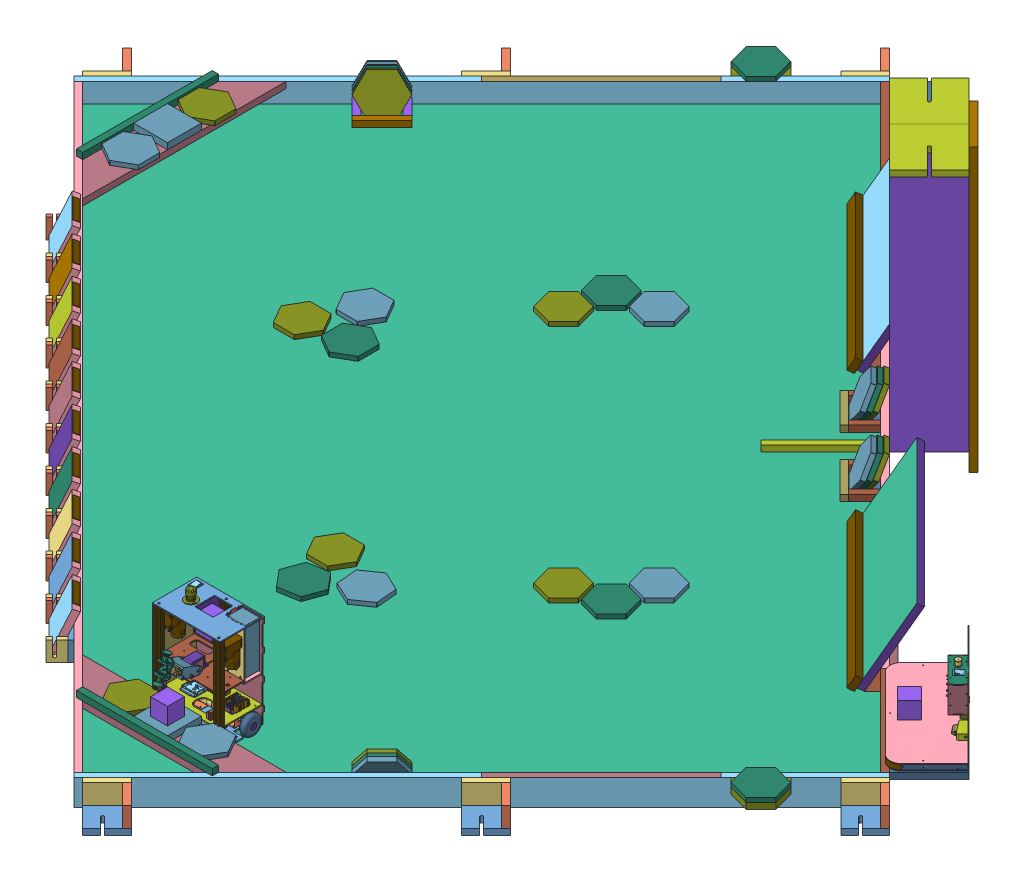
SolidWorks assembly Farid, configuration Default. Lengths in mm.
Overall size (3989.67 1029.4 3989.67).
427 component instances, 139 part files, 92 mates.
Components (placement in the parent):
- robot_sghyr-1: robot_sghyr [Default] at (76.8159 -4.9036 482.9829) x (0 0 1) z (0 1 0) size (182.75 247 92.25) (flexible)
  - base_robot_sghyr-1: base_robot_sghyr [Default] at (64.264 97.0127 214.7631) size (170 240 5)
  - 37 mm DC Geared Motor Mounting Bracket-1: 37 mm DC Geared Motor Mounting Bracket [Default] at (24.264 176.3252 247.7631) x (0 -1 0) z (-1 0 0) size (41 48 40)
  - pololu-37D-encoder-1: pololu-37D-encoder [Default] at (24.264 150.5252 247.7631) x (0 0 -1) z (0 1 0) size (36.8 36.8 92.61)
  - Robot2015_support bille porteuse-1: Robot2015_support bille porteuse [Défaut] at (126.764 97.0127 219.7631) x (-0.866025 -0.5 0) z (-0.5 0.866025 0) size (49.64 16.2 45)
  - 37 mm DC Geared Motor Mounting Bracket-3: 37 mm DC Geared Motor Mounting Bracket [Default] at (24.264 17.7002 247.7631) x (0 1 0) z (1 0 0) size (41 48 40)
  - pololu-37D-encoder-4: pololu-37D-encoder [Default] at (24.264 43.5002 247.7631) x (0 0 -1) z (0 -1 0) size (36.8 36.8 92.61)
  - Arduino Mega 2560.step-1: Arduino Mega 2560.step [Default] at (36.414 47.7208 285.4141) x (-1 0 0) z (0 0 -1) size (107.95 53.42 12.95)
  - Roulement_d3xd10xe4-1: Roulement_d3xd10xe4 [Défaut] at (146.264 -19.9873 225.0631) x (0 0 1) z (-1 0 0) size (5 13 13)
  - etage electronique-1: etage electronique [Default] at (64.264 97.0127 279.7631) x (0 -1 0) z (0 0 1) size (232 153 4)
  - XL4016E1 8A Buck Converter.STEP-1: XL4016E1 8A Buck Converter.STEP [Default] at (36.914 174.7627 283.7631) x (1 0 0) z (0 -1 0) size (65.3 28.6 46.4)
    - 8A Buck Converter PCB.STEP-1: 8A Buck Converter PCB.STEP [Default] at origin size (65.3 1.67 36.5)
    - Heat Exchanger.STEP-1: Heat Exchanger.STEP [Default] at (0 1.65 23.2) size (46 25.1 10.55)
    - Heat Exchanger.STEP-2: Heat Exchanger.STEP [Default] at (0 1.65 -23.2) x (-1 0 0) z (0 0 -1) size (46 25.1 10.55)
    - LargeGreen1000uF 35V Electrolytic Capacitor.STEP-1: LargeGreen1000uF 35V Electrolytic Capacitor.STEP [Default] at (-17.6782 1.65 7.8366) x (0 0 -1) z (1 0 0) size (9.9 26.01 9.9)
    - LargeGreen1000uF 35V Electrolytic Capacitor.STEP-2: LargeGreen1000uF 35V Electrolytic Capacitor.STEP [Default] at (-8.0317 1.65 5.0694) x (0 0 -1) z (1 0 0) size (9.9 26.01 9.9)
    - LargeGreen470uF 35V Electrolytic Capacitor.STEP-1: LargeGreen470uF 35V Electrolytic Capacitor.STEP [Default] at (-17.6617 1.65 -7.7514) x (0 0 1) z (-1 0 0) size (9.9 26.01 9.9)
    - LargeGreen470uF 35V Electrolytic Capacitor.STEP-2: LargeGreen470uF 35V Electrolytic Capacitor.STEP [Default] at (-7.9869 1.65 -5.0151) x (0 0 1) z (-1 0 0) size (9.9 26.01 9.9)
    - Screw Terminal x2.STEP-1: Screw Terminal x2.STEP [Default] at (-9.5 0 12.7839) x (-1 0 0) z (0 0 -1) size (7.95 12.9 10)
    - Screw Terminal x2.STEP-2: Screw Terminal x2.STEP [Default] at (-9.5 0 2.7839) x (-1 0 0) z (0 0 -1) size (7.95 12.9 10)
    - TrimmerW103.STEP-1: TrimmerW103.STEP [Default] at (32.65 6.9 -4.9563) x (0 0 1) z (-1 0 0) size (9.5 15.15 4.8)
    - TrimmerW103.STEP-2: TrimmerW103.STEP [Default] at (32.65 6.9 5.0581) x (0 0 1) z (-1 0 0) size (9.5 15.15 4.8)
    - whiteLEDShortLeed.STEP-1: whiteLEDShortLeed.STEP [Default] at (-13.9989 2.65 -0.1564) x (-1 0 0) z (0 0 -1) size (3.4 13.35 3.4)
    - Schottky Diode 20A 45V STPS2045CT.STEP-1: Schottky Diode 20A 45V STPS2045CT.STEP [Default] at (-0.0419 13.7002 12.65) x (-0.999962 0.008727 0) z (-0.008727 -0.999962 0) size (10.22 3.95 22.6)
    - XL4016E1 8A Voltage Regulator.STEP-1: XL4016E1 8A Voltage Regulator.STEP [Default] at (0 13.7 -12.65) x (1 0 0) z (0 -1 0) size (10.22 3.95 22.6)
    - Coil for Convertor.STEP-1: Coil for Convertor.STEP [Default] at (14.3115 2.9157 0.0112) size (27.99 14.39 26.86)
    - Small Plastic Washer.STEP-1: Small Plastic Washer.STEP [Default] at (0 18.5 -11.95) x (1 0 0) z (0 -1 0) size (6.1 1 6.1)
    - Small Plastic Washer.STEP-2: Small Plastic Washer.STEP [Default] at (0 18.5 10.95) x (1 0 0) z (0 -1 0) size (6.1 1 6.1)
    - pan head cross recess screw_iso_ISO 7045 - M3 x 8 - Z - 8S.STEP-1: pan head cross recess screw_iso_ISO 7045 - M3 x 8 - Z - 8S.STEP [Default] at (0 18.5 -8.55) x (0 0 -1) z (0.923728 0.383049 0) size (10.36 5.6 5.6)
    - pan head cross recess screw_iso_ISO 7045 - M3 x 8 - Z - 8S.STEP-2: pan head cross recess screw_iso_ISO 7045 - M3 x 8 - Z - 8S.STEP [Default] at (0 18.5 8.55) x (0 0 1) z (-1 0 0) size (10.36 5.6 5.6)
    - 1.7mmSmdCeramicCapacitorbrown.STEP-1: 1.7mmSmdCeramicCapacitorbrown.STEP [Default] at (2.849 0.0574 -8.3522) x (-1 0 0) z (0 0 1) size (2.02 0.49 1.04)
    - smdChip8pin.STEP-1: smdChip8pin.STEP [Default] at (19.9049 -0.725 7.6791) x (1 0 0) z (0 0 -1) size (7.3 1.22 4.5)
    - tinyVoltageRegulator.STEP-1: tinyVoltageRegulator.STEP [Default] at (13.3487 0 4.1964) x (-1 0 0) z (0 0 1) size (2.75 0.7 2.1)
    - tinyVoltageRegulator.STEP-2: tinyVoltageRegulator.STEP [Default] at (20.3011 0 11.2685) x (0.999962 0 0.008727) z (0.008727 0 -0.999962) size (2.75 0.7 2.1)
    - TinyVoltageRegulatorAMS1112.STEP-1: TinyVoltageRegulatorAMS1112.STEP [Default] at (15.0739 0.203 -4.8321) x (0 0 -1) z (-1 0 0) size (4.07 1.22 4.96)
    - tinySMDResistor222.STEP-1: tinySMDResistor222.STEP [Default] at (21.8501 0.1177 -6.1765) x (0 0 -1) z (-1 0 0) size (1.52 0.38 0.79)
    - tinySMDResistor.STEP-1: tinySMDResistor.STEP [Default] at (19.9225 0.1177 -6.1853) x (0 0 -1) z (-1 0 0) size (1.52 0.37 0.79)
    - 1.7mmSmdCeramicCapacitorbrown.STEP-2: 1.7mmSmdCeramicCapacitorbrown.STEP [Default] at (24.1073 0.0574 -6.3061) x (0 0 -1) z (-1 0 0) size (2.02 0.49 1.04)
    - 1.7mmSmdCeramicCapacitorbrown.STEP-3: 1.7mmSmdCeramicCapacitorbrown.STEP [Default] at (16.3262 0.0574 0.9562) x (0 0 -1) z (-1 0 0) size (2.02 0.49 1.04)
    - 1.7mmSmdCeramicCapacitorbrown.STEP-4: 1.7mmSmdCeramicCapacitorbrown.STEP [Default] at (18.1093 0.0574 0.9562) x (0 0 -1) z (-1 0 0) size (2.02 0.49 1.04)
    - tinySMDResistor.STEP-2: tinySMDResistor.STEP [Default] at (19.9874 0.1177 1.1419) x (0 0 -1) z (-1 0 0) size (1.52 0.37 0.79)
    - tinySMDResistor.STEP-3: tinySMDResistor.STEP [Default] at (21.6733 0.1177 1.1419) x (0 0 -1) z (-1 0 0) size (1.52 0.37 0.79)
    - tinySMDResistor.STEP-4: tinySMDResistor.STEP [Default] at (23.3916 0.1177 1.1419) x (0 0 -1) z (-1 0 0) size (1.52 0.37 0.79)
    - 1.7mmSmdCeramicCapacitorbrown.STEP-5: 1.7mmSmdCeramicCapacitorbrown.STEP [Default] at (25.4211 0.0574 4.0139) x (0 0 -1) z (-1 0 0) size (2.02 0.49 1.04)
    - 1.7mmSmdCeramicCapacitorbrown.STEP-6: 1.7mmSmdCeramicCapacitorbrown.STEP [Default] at (27.3088 0.0574 4.0139) x (0 0 -1) z (-1 0 0) size (2.02 0.49 1.04)
    - 1.7mmSmdCeramicCapacitorbrown.STEP-7: 1.7mmSmdCeramicCapacitorbrown.STEP [Default] at (23.1777 0.0574 11.1322) x (0 0 -1) z (-1 0 0) size (2.02 0.49 1.04)
    - 1.7mmSmdCeramicCapacitorbrown.STEP-8: 1.7mmSmdCeramicCapacitorbrown.STEP [Default] at (20.6839 0.0574 9.112) x (-0.999962 0 -0.008727) z (-0.008727 0 0.999962) size (2.02 0.49 1.04)
    - tinySMDResistor.STEP-5: tinySMDResistor.STEP [Default] at (17.7351 0.1177 11.3427) x (0 0 -1) z (-1 0 0) size (1.52 0.37 0.79)
    - tinySMDResistor.STEP-6: tinySMDResistor.STEP [Default] at (16.0827 0.1177 11.3427) x (0 0 -1) z (-1 0 0) size (1.52 0.37 0.79)
    - tinySMDResistor.STEP-7: tinySMDResistor.STEP [Default] at (16.906 0.1177 9.0199) x (-0.999962 0 -0.008727) z (-0.008727 0 0.999962) size (1.52 0.37 0.79)
    - tinySMDResistor.STEP-8: tinySMDResistor.STEP [Default] at (25.3907 0.1177 9.8144) x (-0.999962 0 -0.008727) z (-0.008727 0 0.999962) size (1.52 0.37 0.79)
    - R010 Resistor SMD.STEP-1: R010 Resistor SMD.STEP [Default] at (-19.919 0 5.2469) x (0 0 -1) z (-1 0 0) size (6.7 0.52 3.1)
    - solder.STEP-1: solder.STEP [Default] at (-27.65 0 -7.4411) x (-0.837169 0 -0.546944) z (-0.546944 0 0.837169) size (1.17 0.65 1.17)
    - solder.STEP-2: solder.STEP [Default] at (-27.65 0 -2.711) x (-0.837169 0 -0.546944) z (-0.546944 0 0.837169) size (1.17 0.65 1.17)
    - solder.STEP-3: solder.STEP [Default] at (-27.65 0 2.537) x (-0.837169 0 -0.546944) z (-0.546944 0 0.837169) size (1.17 0.65 1.17)
    - solder.STEP-4: solder.STEP [Default] at (-27.65 0 7.3016) x (-0.837169 0 -0.546944) z (-0.546944 0 0.837169) size (1.17 0.65 1.17)
    - solder1.8.STEP-1: solder1.8.STEP [Default] at (-20.8987 0 -15.5519) x (-0.837169 0 -0.546944) z (-0.546944 0 0.837169) size (1.8 0.65 1.8)
    - solder1.8.STEP-2: solder1.8.STEP [Default] at (20.8325 0 -15.5519) x (-0.837169 0 -0.546944) z (-0.546944 0 0.837169) size (1.8 0.65 1.8)
    - solder1.8.STEP-3: solder1.8.STEP [Default] at (20.8325 0 15.5391) x (-0.837169 0 -0.546944) z (-0.546944 0 0.837169) size (1.8 0.65 1.8)
    - solder1.8.STEP-4: solder1.8.STEP [Default] at (-20.8987 0 15.5391) x (-0.837169 0 -0.546944) z (-0.546944 0 0.837169) size (1.8 0.65 1.8)
    - solder.STEP-5: solder.STEP [Default] at (30.4698 0 7.6228) x (-0.837169 0 -0.546944) z (-0.546944 0 0.837169) size (1.17 0.65 1.17)
    - solder.STEP-6: solder.STEP [Default] at (30.4698 0 2.537) x (-0.837169 0 -0.546944) z (-0.546944 0 0.837169) size (1.17 0.65 1.17)
    - solder.STEP-7: solder.STEP [Default] at (30.4698 0 -2.454) x (-0.837169 0 -0.546944) z (-0.546944 0 0.837169) size (1.17 0.65 1.17)
    - solder.STEP-8: solder.STEP [Default] at (30.4698 0 -7.4732) x (-0.837169 0 -0.546944) z (-0.546944 0 0.837169) size (1.17 0.65 1.17)
    - solder.STEP-9: solder.STEP [Default] at (30.4698 0 -4.9355) x (-0.837169 0 -0.546944) z (-0.546944 0 0.837169) size (1.17 0.65 1.17)
    - solder.STEP-10: solder.STEP [Default] at (30.4698 0 5.0529) x (-0.837169 0 -0.546944) z (-0.546944 0 0.837169) size (1.17 0.65 1.17)
    - solder1.8.STEP-5: solder1.8.STEP [Default] at (1.0959 0 2.1506) x (-0.837169 0 -0.546944) z (-0.546944 0 0.837169) size (1.8 0.65 1.8)
    - solder1.8.STEP-6: solder1.8.STEP [Default] at (8.9457 0 2.3519) x (-0.837169 0 -0.546944) z (-0.546944 0 0.837169) size (1.8 0.65 1.8)
    - solder.STEP-11: solder.STEP [Default] at (-3.9931 0 -10.2017) x (-0.837169 0 -0.546944) z (-0.546944 0 0.837169) size (1.17 0.65 1.17)
    - solder.STEP-12: solder.STEP [Default] at (-1.9931 0 -10.2017) x (-0.837169 0 -0.546944) z (-0.546944 0 0.837169) size (1.17 0.65 1.17)
    - solder.STEP-13: solder.STEP [Default] at (0.0069 0 -10.2017) x (-0.837169 0 -0.546944) z (-0.546944 0 0.837169) size (1.17 0.65 1.17)
    - solder.STEP-14: solder.STEP [Default] at (2.0069 0 -10.2017) x (-0.837169 0 -0.546944) z (-0.546944 0 0.837169) size (1.17 0.65 1.17)
    - solder.STEP-15: solder.STEP [Default] at (4.0069 0 -10.2017) x (-0.837169 0 -0.546944) z (-0.546944 0 0.837169) size (1.17 0.65 1.17)
    - solder.STEP-16: solder.STEP [Default] at (-2.7433 0 10.0764) x (-0.873283 0 -0.487214) z (-0.487214 0 0.873283) size (1.17 0.65 1.17)
    - solder.STEP-17: solder.STEP [Default] at (-0.2033 0 10.0764) x (-0.873283 0 -0.487214) z (-0.487214 0 0.873283) size (1.17 0.65 1.17)
    - solder.STEP-18: solder.STEP [Default] at (2.3367 0 10.0764) x (-0.873283 0 -0.487214) z (-0.487214 0 0.873283) size (1.17 0.65 1.17)
    - solder.STEP-19: solder.STEP [Default] at (-8.0296 0 7.8897) x (-0.873283 0 -0.487214) z (-0.487214 0 0.873283) size (1.17 0.65 1.17)
    - solder.STEP-20: solder.STEP [Default] at (-8.0296 0 2.259) x (-0.873283 0 -0.487214) z (-0.487214 0 0.873283) size (1.17 0.65 1.17)
    - solder.STEP-21: solder.STEP [Default] at (-8.0296 0 -2.2341) x (-0.873283 0 -0.487214) z (-0.487214 0 0.873283) size (1.17 0.65 1.17)
    - solder.STEP-22: solder.STEP [Default] at (-8.0296 0 -7.8634) x (-0.873283 0 -0.487214) z (-0.487214 0 0.873283) size (1.17 0.65 1.17)
    - solder.STEP-23: solder.STEP [Default] at (-17.6872 0 -10.549) x (-0.873283 0 -0.487214) z (-0.487214 0 0.873283) size (1.17 0.65 1.17)
    - solder.STEP-24: solder.STEP [Default] at (-17.6872 0 -4.9388) x (-0.873283 0 -0.487214) z (-0.487214 0 0.873283) size (1.17 0.65 1.17)
    - solder.STEP-25: solder.STEP [Default] at (-17.6872 0 10.6333) x (-0.873283 0 -0.487214) z (-0.487214 0 0.873283) size (1.17 0.65 1.17)
    - solder.STEP-26: solder.STEP [Default] at (-17.6872 0 5.0231) x (-0.873283 0 -0.487214) z (-0.487214 0 0.873283) size (1.17 0.65 1.17)
    - solder.STEP-27: solder.STEP [Default] at (-15.2798 0 -0.193) x (-0.873283 0 -0.487214) z (-0.487214 0 0.873283) size (1.17 0.65 1.17)
    - solder.STEP-28: solder.STEP [Default] at (-12.7921 0 -0.193) x (-0.873283 0 -0.487214) z (-0.487214 0 0.873283) size (1.17 0.65 1.17)
  - Roulement_d3xd10xe4-3: Roulement_d3xd10xe4 [Défaut] at (146.264 214.0127 225.0631) x (0 0 1) z (1 0 0) size (5 13 13)
- étage 3-1: étage 3 [Default] at (169.8286 379.2835 544.2469) x (0 0 1) z (-1 0 0) size (162 4 232)
- Servo Motor MG996R _米字摇臂.step-3: Servo Motor MG996R _米字摇臂.step [Default] at (167.7867 421.7628 658.2361) x (-1 0 0) z (0 0.938295 -0.345835) size (56.95 44.55 19.71)
- Servo-1: Servo [Défaut] at (182.7867 399.2835 587.7469) x (0 -1 0) z (-1 0 0) size (32 43 41.5)
- bras_replique-1: bras_replique [Default] at (141.7867 399.2835 597.2469) x (0 0.345835 0.938295) z (1 0 0) size (77.5 32 70)
- SUPPORT VENTOUSE-1: SUPPORT VENTOUSE [Default] at (157.6946 426.1895 670.2462) x (0 0.938295 -0.345835) z (0 0.345835 0.938295) size (60 44.83 4)
- Access_HS-645_BrasRondPetitModele-1: Access_HS-645_BrasRondPetitModele [Défaut] at (157.6946 428.4796 668.8693) x (1 0 0) z (0 -0.938295 0.345835) size (24 5 24)
- support servo kbyr-1: support servo kbyr [Default] at (181.5367 383.2835 548.2469) x (0 0 1) z (-1 0 0) size (79 38 30)
- PompeVide-AirpoD2028B-12vdc-1: PompeVide-AirpoD2028B-12vdc [Défaut] at (270.3286 514.8594 552.1469) x (1 0 0) z (0 -1 0) size (38.6 62.4 92)
- TABLE_2021.step-1: TABLE_2021.step [Default] at (-533.2781 201.1947 -2548.6626) x (0.707107 0 0.707107) z (0 1 0) size (3306.25 2336 1029.4)
  - BaseTable.step-1: BaseTable.step [Default] at (0 0 -22) x (1 0 0) z (0 -1 0) size (3288 1022 2266)
    - Edge Beacon Right.step-1: Edge Beacon Right.step [Default] at (-884.0915 354.4211 0) x (1 0 0) z (0 1 0) size (122 122 92)
      - EdgeBeacons_Base.step-1: EdgeBeacons_Base.step [Default] at (3967.0915 -989 -332.4211) x (0 -1 0) z (1 0 0) size (122 22 122)
      - EdgeBeacons_SmallBorder.step-1: EdgeBeacons_SmallBorder.step [Default] at (4028.0915 -950 -332.4211) x (0 1 0) z (1 0 0) size (22 70 100)
      - EdgeBeacons_LargeBorder.step-1: EdgeBeacons_LargeBorder.step [Default] at (3906.0915 -1050 -332.4211) x (1 0 0) z (0 -1 0) size (22 70 122)
    - Edge Beacon Left.step-1: Edge Beacon Left.step [Default] at (-1609.4995 44.4467 0) x (1 0 0) z (0 1 0) size (122 122 92)
      - EdgeBeacons_Base.step-1: EdgeBeacons_Base.step [Default] at (1526.4995 -39 -44.4467) x (0 -1 0) z (-1 0 0) size (122 22 122)
      - EdgeBeacons_LargeBorder.step-1: EdgeBeacons_LargeBorder.step [Default] at (1565.4995 -100 -22.4467) x (1 0 0) z (0 -1 0) size (22 70 122)
      - EdgeBeacons_SmallBorder.step-1: EdgeBeacons_SmallBorder.step [Default] at (1465.4995 22 -22.4467) x (0 -1 0) z (-1 0 0) size (22 70 100)
    - Edge Beacon Right_1.step-1: Edge Beacon Right_1.step [Default] at (-884.0915 354.4211 0) x (1 0 0) z (0 1 0) size (122 122 92)
      - EdgeBeacons_Base.step-1: EdgeBeacons_Base.step [Default] at (3967.0915 -39 -332.4211) x (0 -1 0) z (1 0 0) size (122 22 122)
      - EdgeBeacons_SmallBorder.step-1: EdgeBeacons_SmallBorder.step [Default] at (4028.0915 0 -332.4211) x (0 1 0) z (1 0 0) size (22 70 100)
      - EdgeBeacons_LargeBorder.step-1: EdgeBeacons_LargeBorder.step [Default] at (3906.0915 -100 -332.4211) x (1 0 0) z (0 -1 0) size (22 70 122)
    - Edge Beacon Right_2.step-1: Edge Beacon Right_2.step [Default] at (-1546.4323 1056.5508 0) x (1 0 0) z (0 1 0) size (122 122 92)
      - EdgeBeacons_Base.step-1: EdgeBeacons_Base.step [Default] at (4629.4323 -1939 -1034.5508) x (0 -1 0) z (1 0 0) size (122 22 122)
      - EdgeBeacons_SmallBorder.step-1: EdgeBeacons_SmallBorder.step [Default] at (4690.4323 -1900 -1034.5508) x (0 1 0) z (1 0 0) size (22 70 100)
      - EdgeBeacons_LargeBorder.step-1: EdgeBeacons_LargeBorder.step [Default] at (4568.4323 -2000 -1034.5508) x (1 0 0) z (0 -1 0) size (22 70 122)
    - Edge Beacon Left_1.step-1: Edge Beacon Left_1.step [Default] at (-933.7648 1396.3534 0) x (1 0 0) z (0 1 0) size (122 122 92)
      - EdgeBeacons_Base.step-1: EdgeBeacons_Base.step [Default] at (850.7648 -1939 -1396.3534) x (0 -1 0) z (-1 0 0) size (122 22 122)
      - EdgeBeacons_LargeBorder.step-1: EdgeBeacons_LargeBorder.step [Default] at (889.7648 -2000 -1374.3534) x (1 0 0) z (0 -1 0) size (22 70 122)
      - EdgeBeacons_SmallBorder.step-1: EdgeBeacons_SmallBorder.step [Default] at (789.7648 -1878 -1374.3534) x (0 -1 0) z (-1 0 0) size (22 70 100)
    - Edge Beacon Left_2.step-1: Edge Beacon Left_2.step [Default] at (-2304.4911 1279.1137 0) x (1 0 0) z (0 1 0) size (122 122 92)
      - EdgeBeacons_Base.step-1: EdgeBeacons_Base.step [Default] at (2221.4911 -989 -1279.1137) x (0 -1 0) z (-1 0 0) size (122 22 122)
      - EdgeBeacons_LargeBorder.step-1: EdgeBeacons_LargeBorder.step [Default] at (2260.4911 -1050 -1257.1137) x (1 0 0) z (0 -1 0) size (22 70 122)
      - EdgeBeacons_SmallBorder.step-1: EdgeBeacons_SmallBorder.step [Default] at (2160.4911 -928 -1257.1137) x (0 -1 0) z (-1 0 0) size (22 70 100)
    - BorderLong.step-1: BorderLong.step [Default] at (0 0 -22) size (3000 92 22)
    - BorderLong.step-2: BorderLong.step [Default] at (3000 0 2022) x (-1 0 0) z (0 0 -1) size (3000 92 22)
    - BorderSmall.step-1: BorderSmall.step [Default] at (-22 0 2022) x (0 0 -1) z (1 0 0) size (2044 92 22)
    - BorderSmall.step-2: BorderSmall.step [Default] at (3022 0 -22) x (0 0 1) z (-1 0 0) size (2044 92 22)
    - Ground.step-1: Ground.step [Default] at origin size (3000 22 2000)
    - MiddleBeaconTop.step-1: MiddleBeaconTop.step [Default] at (1500 22 -122) size (400 22 200)
    - MiddleBeaconVertSupport1.step-1: MiddleBeaconVertSupport1.step [Default] at (1500 22 -22) x (0 0 1) z (-1 0 0) size (200 978 22)
    - MiddleBeaconVertSupport2.step-1: MiddleBeaconVertSupport2.step [Default] at (1600 22 -233) size (200 1000 22)
    - ExperimentZone.step-1: ExperimentZone.step [Default] at (225 92 -22) size (450 22 200)
    - ExperimentZone.step-2: ExperimentZone.step [Default] at (2775 92 -22) size (450 22 200)
    - PaintExperience.step-1: PaintExperience.step [Default] at (0 92 -22) size (450 0.1 22)
    - PaintExperience.step-2: PaintExperience.step [Default] at (2550 92 -22) size (450 0.1 22)
    - BaseTable-0.step-1: BaseTable-0.step [Default] at origin size (22 0.1 600)
    - BaseTable-1.step-1: BaseTable-1.step [Default] at origin size (22 0.1 600)
  - Echantillons.step-1: Echantillons.step [Default] at origin size (3292.15 1762.13 85)
    - EchantillonBleu.step-1: EchantillonBleu.step [Default] at (900 -555 0) x (0.5 0.866025 0) z (0 0 1) size (129.9 149.69 15)
    - EchantillonBleu.step-2: EchantillonBleu.step [Default] at (892.3031 -1292.3031 15) x (0.965926 0.258819 0) z (0 0 -1) size (129.9 149.69 15)
    - EchantillonBleu.step-3: EchantillonBleu.step [Default] at (2100 -555 0) x (0.5 0.866025 0) z (0 0 1) size (129.9 149.69 15)
    - EchantillonBleu.step-4: EchantillonBleu.step [Default] at (2113.9218 -1288.3769 15) x (0.34202 -0.939693 0) z (0 0 -1) size (129.9 149.69 15)
    - EchantillonVert.step-1: EchantillonVert.step [Default] at (2085.0581 -1446.2787 15) x (0.906308 0.422618 0) z (0 0 -1) size (129.9 149.69 15)
    - EchantillonRouge.step-1: EchantillonRouge.step [Default] at (1954.3221 -1366.4789 15) x (0.258819 0.965926 0) z (0 0 -1) size (129.9 149.69 15)
    - EchantillonVert.step-2: EchantillonVert.step [Default] at (830 -675 0) x (0.5 0.866025 0) z (0 0 1) size (129.9 149.69 15)
    - EchantillonRouge.step-2: EchantillonRouge.step [Default] at (900 -795 0) x (0.5 0.866025 0) z (0 0 1) size (129.9 149.69 15)
    - EchantillonVert.step-3: EchantillonVert.step [Default] at (2170 -675 0) x (0.5 0.866025 0) z (0 0 1) size (129.9 149.69 15)
    - EchantillonRouge.step-3: EchantillonRouge.step [Default] at (2100 -795 0) x (0.5 0.866025 0) z (0 0 1) size (129.9 149.69 15)
    - EchantillonVert.step-4: EchantillonVert.step [Default] at (1044.2641 -1329.1257 15) x (0.965926 -0.258819 0) z (0 0 -1) size (129.9 149.69 15)
    - EchantillonRouge.step-4: EchantillonRouge.step [Default] at (950 -1450 15) x (0.965926 0.258819 0) z (0 0 -1) size (129.9 149.69 15)
    - EchantillonBleu.step-5: EchantillonBleu.step [Default] at (311.5685 -1879.3503 70) x (0.258819 -0.965926 0) z (0 0 1) size (129.9 149.69 15)
    - EchantillonRouge.step-5: EchantillonRouge.step [Default] at (120.6497 -1688.4315 70) x (-0.258819 0.965926 0) z (0 0 1) size (129.9 149.69 15)
    - EchantillonBleu.step-6: EchantillonBleu.step [Default] at (2879.3503 -1688.4315 70) x (0.965926 0.258819 0) z (0 0 1) size (129.9 149.69 15)
    - EchantillonRouge.step-6: EchantillonRouge.step [Default] at (2688.4315 -1879.3503 70) x (-0.965926 -0.258819 0) z (0 0 1) size (129.9 149.69 15)
    - EchantillonVert.step-5: EchantillonVert.step [Default] at (-64.9519 -300 70) x (-0.5 0.866025 0) z (0 0 1) size (129.9 149.69 15)
    - EchantillonVert.step-6: EchantillonVert.step [Default] at (3064.9519 -300 70) size (129.9 149.69 15)
  - Frises.step-1: Frises.step [Default] at origin size (2100 194.46 292.81)
    - FriseJaune.step-1: FriseJaune.step [Default] at (810 0 0) x (0 -1 0) z (0 0 1) size (194.46 720 292.81)
      - Frise.step-1: Frise.step [Default] at origin size (194.46 720 292.81)
        - FRISE_2.step-1: FRISE_2.step [Default] at origin size (169.05 720 270.81)
        - BORDURE.step-1: BORDURE.step [Default] at origin size (41.05 720 49.11)
        - TRIANGLE_GAUCHE.step-1: TRIANGLE_GAUCHE.step [Default] at origin size (40.41 22 70)
        - TRIANGLE_DROIT.step-1: TRIANGLE_DROIT.step [Default] at origin size (40.41 22 70)
        - TRIANGLE_CENTRE.step-1: TRIANGLE_CENTRE.step [Default] at origin size (40.41 22 70)
        - TaquetArriere.step-1: TaquetArriere.step [Default] at origin size (22 22 168.21)
        - TaquetArriere.step-2: TaquetArriere.step [Default] at (0 698 0) size (22 22 168.21)
        - TaquetArriere.step-3: TaquetArriere.step [Default] at (0 349 0) size (22 22 168.21)
      - FriseJaune-2.step-1: FriseJaune-2.step [Default] at origin size (150.01 720 259.81)
    - FriseViolet.step-1: FriseViolet.step [Default] at (2190 0 0) x (0 -1 0) z (0 0 1) size (194.46 720 292.81)
      - Frise_1.step-1: Frise_1.step [Default] at origin size (194.46 720 292.81)
        - FRISE_2.step-1: FRISE_2.step [Default] at origin size (169.05 720 270.81)
        - BORDURE.step-1: BORDURE.step [Default] at origin size (41.05 720 49.11)
        - TRIANGLE_GAUCHE.step-1: TRIANGLE_GAUCHE.step [Default] at origin size (40.41 22 70)
        - TRIANGLE_DROIT.step-1: TRIANGLE_DROIT.step [Default] at origin size (40.41 22 70)
        - TRIANGLE_CENTRE.step-1: TRIANGLE_CENTRE.step [Default] at origin size (40.41 22 70)
        - TaquetArriere.step-1: TaquetArriere.step [Default] at origin size (22 22 168.21)
        - TaquetArriere.step-2: TaquetArriere.step [Default] at (0 698 0) size (22 22 168.21)
        - TaquetArriere.step-3: TaquetArriere.step [Default] at (0 349 0) size (22 22 168.21)
      - FriseViolet-3.step-1: FriseViolet-3.step [Default] at origin size (150.01 720 259.81)
  - Distributeurs.step-1: Distributeurs.step [Default] at origin size (3259.81 2051.07 183.14)
    - Distributeur 2 Side.step-1: Distributeur 2 Side.step [Default] at (11 -1250 0) x (0 1 0) z (1 0 0) size (187.35 183.14 137.52)
      - TasseauBordure.step-1: TasseauBordure.step [Default] at origin size (106 22 22)
      - TasseauCote.step-1: TasseauCote.step [Default] at (-64 0 29) size (22 22 80)
      - TasseauCote.step-2: TasseauCote.step [Default] at (64 0 29) size (22 22 80)
      - TasseauAvant.step-1: TasseauAvant.step [Default] at (0 0 80) size (150 22 22)
      - EchantillonBleu.step-1: EchantillonBleu.step [Default] at (0 59.0455 -5.9792) x (0.866025 0.454532 -0.208327) z (0 0.416655 0.909065) size (129.9 149.69 15)
      - EchantillonVert.step-1: EchantillonVert.step [Default] at (0 59.0455 10.5213) x (0.866025 0.454532 -0.208327) z (0 0.416655 0.909065) size (129.9 149.69 15)
      - EchantillonRouge.step-1: EchantillonRouge.step [Default] at (0 59.0455 27.0218) x (0.866025 0.454532 -0.208327) z (0 0.416655 0.909065) size (129.9 149.69 15)
    - Distributeur 2 Side_1.step-1: Distributeur 2 Side_1.step [Default] at (2989 -1250 0) x (0 -1 0) z (-1 0 0) size (187.35 183.14 137.52)
      - TasseauBordure.step-1: TasseauBordure.step [Default] at origin size (106 22 22)
      - TasseauCote.step-1: TasseauCote.step [Default] at (-64 0 29) size (22 22 80)
      - TasseauCote.step-2: TasseauCote.step [Default] at (64 0 29) size (22 22 80)
      - TasseauAvant.step-1: TasseauAvant.step [Default] at (0 0 80) size (150 22 22)
      - EchantillonBleu.step-1: EchantillonBleu.step [Default] at (0 59.0455 -5.9792) x (0.866025 0.454532 -0.208327) z (0 0.416655 0.909065) size (129.9 149.69 15)
      - EchantillonVert.step-1: EchantillonVert.step [Default] at (0 59.0455 10.5213) x (0.866025 0.454532 -0.208327) z (0 0.416655 0.909065) size (129.9 149.69 15)
      - EchantillonRouge.step-1: EchantillonRouge.step [Default] at (0 59.0455 27.0218) x (0.866025 0.454532 -0.208327) z (0 0.416655 0.909065) size (129.9 149.69 15)
    - Distributeur 2 Top.step-1: Distributeur 2 Top.step [Default] at (1650 -11 0) x (1 0 0) z (0 -1 0) size (187.35 183.14 137.52)
      - TasseauBordure_1.step-1: TasseauBordure_1.step [Default] at origin size (106 22 22)
      - TasseauCote_1.step-1: TasseauCote_1.step [Default] at (-64 0 29) size (22 22 80)
      - TasseauCote_1.step-2: TasseauCote_1.step [Default] at (64 0 29) size (22 22 80)
      - TasseauAvant_1.step-1: TasseauAvant_1.step [Default] at (0 0 80) size (150 22 22)
      - EchantillonBleu.step-1: EchantillonBleu.step [Default] at (0 59.0455 27.0218) x (0.866025 0.454532 -0.208327) z (0 0.416655 0.909065) size (129.9 149.69 15)
      - EchantillonRouge.step-1: EchantillonRouge.step [Default] at (0 59.0455 -5.9792) x (0.866025 0.454532 -0.208327) z (0 0.416655 0.909065) size (129.9 149.69 15)
      - EchantillonVert.step-1: EchantillonVert.step [Default] at (0 59.0455 10.5213) x (0.866025 0.454532 -0.208327) z (0 0.416655 0.909065) size (129.9 149.69 15)
    - Distributeur 2 Top_1.step-1: Distributeur 2 Top_1.step [Default] at (1350 -11 0) x (1 0 0) z (0 -1 0) size (187.35 183.14 137.52)
      - TasseauBordure_1.step-1: TasseauBordure_1.step [Default] at origin size (106 22 22)
      - TasseauCote_1.step-1: TasseauCote_1.step [Default] at (-64 0 29) size (22 22 80)
      - TasseauCote_1.step-2: TasseauCote_1.step [Default] at (64 0 29) size (22 22 80)
      - TasseauAvant_1.step-1: TasseauAvant_1.step [Default] at (0 0 80) size (150 22 22)
      - EchantillonBleu.step-1: EchantillonBleu.step [Default] at (0 59.0455 27.0218) x (0.866025 0.454532 -0.208327) z (0 0.416655 0.909065) size (129.9 149.69 15)
      - EchantillonRouge.step-1: EchantillonRouge.step [Default] at (0 59.0455 -5.9792) x (0.866025 0.454532 -0.208327) z (0 0.416655 0.909065) size (129.9 149.69 15)
      - EchantillonVert.step-1: EchantillonVert.step [Default] at (0 59.0455 10.5213) x (0.866025 0.454532 -0.208327) z (0 0.416655 0.909065) size (129.9 149.69 15)
    - DistributeurCoin.step-1: DistributeurCoin.step [Default] at (0 -2000 175) size (525.56 525.56 44)
      - Taquet.step-1: Taquet.step [Default] at (0 0 -197) size (510 510 22)
      - SupportStatuette.step-1: SupportStatuette.step [Default] at (0 0 -197) size (169.71 169.71 22)
      - Taquet (1).step-1: Taquet (1).step [Default] at (0 0 -197) size (355.85 355.85 22)
    - DistributeurCoin_1.step-1: DistributeurCoin_1.step [Default] at (3000 -2000 300) x (0 1 0) z (0 0 1) size (525.56 525.56 44)
      - Taquet.step-1: Taquet.step [Default] at (0 0 -322) size (510 510 22)
      - SupportStatuette.step-1: SupportStatuette.step [Default] at (0 0 -322) size (169.71 169.71 22)
      - Taquet (1).step-1: Taquet (1).step [Default] at (0 0 -322) size (355.85 355.85 22)
    - DistributeurBordure.step-1: DistributeurBordure.step [Default] at (-200 -250 0) size (107.9 150 92)
      - Support (1).step-1: Support (1).step [Default] at (200 -50 -22) size (107.9 150 22)
      - Equerre.step-1: Equerre.step [Default] at (200 -50 -22) size (70 22 70)
    - DistributeurBordure_1.step-1: DistributeurBordure_1.step [Default] at (3250 -250 0) x (-1 0 0) z (0 0 1) size (107.9 150 92)
      - Support (1).step-1: Support (1).step [Default] at (250 50 -22) size (107.9 150 22)
      - Equerre.step-1: Equerre.step [Default] at (250 50 -22) size (70 22 70)
  - CarreFouille.step-1: CarreFouille.step [Default] at origin size (1850 85.95 153.3)
    - CarreFouilleTresorJaune.step-1: CarreFouilleTresorJaune.step [Default] at (667.5 -2000 0) x (0 -1 0) z (0 0 1) size (85.95 185 153.3)
      - CarreFouille_1.step-1: CarreFouille_1.step [Default] at (64.8942 -232.3942 0) size (85.94 185 153.3)
        - PCB_datation.step-1: PCB_datation.step [Default] at (0 0 158.7231) x (0 1 0) z (0 0 1) size (100 19.02 9.26)
          - PCB Component.step-1: PCB Component.step [Default] at (232.3942 48.7058 -10.7729) x (1 0 0) z (0 0.390731 0.920505) size (100 20 1.57)
            - Board.step-1: Board.step [Default] at origin size (100 20 1.57)
        - BASE.step-1: BASE.step [Default] at (-27.8942 232.3942 35) size (15 185 70)
        - LEFT_ARM.step-1: LEFT_ARM.step [Default] at (-27.8942 232.3942 35) size (55 15 70)
        - RIGHT_ARM.step-1: RIGHT_ARM.step [Default] at (-27.8942 232.3942 35) size (55 15 70)
        - SQUARE.step-1: SQUARE.step [Default] at (-31.092 232.3942 20.7181) x (0.920505 0 0.390731) z (-0.390731 0 0.920505) size (22 150 150)
      - CarreFouilleTresorJaune-4.step-1: CarreFouilleTresorJaune-4.step [Default] at origin size (58.62 150 138.08)
      - CarreFouilleTresorJaune-5.step-1: CarreFouilleTresorJaune-5.step [Default] at origin size (58.62 150 138.08)
    - CarreFouilleRadioactif.step-1: CarreFouilleRadioactif.step [Default] at (1037.5 -2000 0) x (0 -1 0) z (0 0 1) size (85.95 185 153.3)
      - CarreFouille_2.step-1: CarreFouille_2.step [Default] at (364.8942 -102.3942 0) size (85.94 185 153.3)
        - PCB_datation_1.step-1: PCB_datation_1.step [Default] at (0 0 158.7231) x (0 1 0) z (0 0 1) size (100 19.02 9.26)
          - PCB Component_1.step-1: PCB Component_1.step [Default] at (102.3942 348.7058 -10.7729) x (1 0 0) z (0 0.390731 0.920505) size (100 20 1.57)
            - Board.step-1: Board.step [Default] at origin size (100 20 1.57)
        - BASE.step-1: BASE.step [Default] at (-327.8942 102.3942 35) size (15 185 70)
        - LEFT_ARM.step-1: LEFT_ARM.step [Default] at (-327.8942 102.3942 35) size (55 15 70)
        - RIGHT_ARM.step-1: RIGHT_ARM.step [Default] at (-327.8942 102.3942 35) size (55 15 70)
        - SQUARE.step-1: SQUARE.step [Default] at (-331.092 102.3942 20.7181) x (0.920505 0 0.390731) z (-0.390731 0 0.920505) size (22 150 150)
      - CarreFouilleRadioactif-6.step-1: CarreFouilleRadioactif-6.step [Default] at origin size (58.62 150 138.08)
      - CarreFouilleRadioactif-7.step-1: CarreFouilleRadioactif-7.step [Default] at origin size (58.62 150 138.08)
    - CarreFouilleTresorJaune_1.step-1: CarreFouilleTresorJaune_1.step [Default] at (852.5 -2000 0) x (0 -1 0) z (0 0 1) size (85.95 185 153.3)
      - CarreFouille_3.step-1: CarreFouille_3.step [Default] at (264.8942 282.6058 0) size (85.94 185 153.3)
        - PCB_datation_2.step-1: PCB_datation_2.step [Default] at (0 0 158.7231) x (0 1 0) z (0 0 1) size (100 19.02 9.26)
          - PCB Component_2.step-1: PCB Component_2.step [Default] at (-282.6058 248.7058 -10.7729) x (1 0 0) z (0 0.390731 0.920505) size (100 20 1.57)
            - Board.step-1: Board.step [Default] at origin size (100 20 1.57)
        - BASE.step-1: BASE.step [Default] at (-227.8942 -282.6058 35) size (15 185 70)
        - LEFT_ARM.step-1: LEFT_ARM.step [Default] at (-227.8942 -282.6058 35) size (55 15 70)
        - RIGHT_ARM.step-1: RIGHT_ARM.step [Default] at (-227.8942 -282.6058 35) size (55 15 70)
        - SQUARE.step-1: SQUARE.step [Default] at (-231.092 -282.6058 20.7181) x (0.920505 0 0.390731) z (-0.390731 0 0.920505) size (22 150 150)
      - CarreFouilleTresorJaune_1-8.step-1: CarreFouilleTresorJaune_1-8.step [Default] at origin size (58.62 150 138.08)
      - CarreFouilleTresorJaune_1-9.step-1: CarreFouilleTresorJaune_1-9.step [Default] at origin size (58.62 150 138.08)
    - CarreFouilleTresorViolet.step-1: CarreFouilleTresorViolet.step [Default] at (1222.5 -2000 0) x (0 -1 0) z (0 0 1) size (85.95 185 153.3)
      - CarreFouille_4.step-1: CarreFouille_4.step [Default] at (464.8942 112.6058 0) size (85.94 185 153.3)
        - PCB_datation_3.step-1: PCB_datation_3.step [Default] at (0 0 158.7231) x (0 1 0) z (0 0 1) size (100 19.02 9.26)
          - PCB Component_3.step-1: PCB Component_3.step [Default] at (-112.6058 448.7058 -10.7729) x (1 0 0) z (0 0.390731 0.920505) size (100 20 1.57)
            - Board.step-1: Board.step [Default] at origin size (100 20 1.57)
        - BASE.step-1: BASE.step [Default] at (-427.8942 -112.6058 35) size (15 185 70)
        - LEFT_ARM.step-1: LEFT_ARM.step [Default] at (-427.8942 -112.6058 35) size (55 15 70)
        - RIGHT_ARM.step-1: RIGHT_ARM.step [Default] at (-427.8942 -112.6058 35) size (55 15 70)
        - SQUARE.step-1: SQUARE.step [Default] at (-431.092 -112.6058 20.7181) x (0.920505 0 0.390731) z (-0.390731 0 0.920505) size (22 150 150)
      - CarreFouilleTresorViolet-10.step-1: CarreFouilleTresorViolet-10.step [Default] at origin size (58.62 150 138.08)
      - CarreFouilleTresorViolet-11.step-1: CarreFouilleTresorViolet-11.step [Default] at origin size (58.62 150 138.08)
    - CarreFouilleTresorJaune_2.step-1: CarreFouilleTresorJaune_2.step [Default] at (1407.5 -2000 0) x (0 -1 0) z (0 0 1) size (85.95 185 153.3)
      - CarreFouille_5.step-1: CarreFouille_5.step [Default] at (464.8942 27.6058 0) size (85.94 185 153.3)
        - PCB_datation_4.step-1: PCB_datation_4.step [Default] at (0 0 158.7231) x (0 1 0) z (0 0 1) size (100 19.02 9.26)
          - PCB Component_4.step-1: PCB Component_4.step [Default] at (-27.6058 448.7058 -10.7729) x (1 0 0) z (0 0.390731 0.920505) size (100 20 1.57)
            - Board.step-1: Board.step [Default] at origin size (100 20 1.57)
        - BASE.step-1: BASE.step [Default] at (-427.8942 -27.6058 35) size (15 185 70)
        - LEFT_ARM.step-1: LEFT_ARM.step [Default] at (-427.8942 -27.6058 35) size (55 15 70)
        - RIGHT_ARM.step-1: RIGHT_ARM.step [Default] at (-427.8942 -27.6058 35) size (55 15 70)
        - SQUARE.step-1: SQUARE.step [Default] at (-431.092 -27.6058 20.7181) x (0.920505 0 0.390731) z (-0.390731 0 0.920505) size (22 150 150)
      - CarreFouilleTresorJaune_2-12.step-1: CarreFouilleTresorJaune_2-12.step [Default] at origin size (58.62 150 138.08)
      - CarreFouilleTresorJaune_2-13.step-1: CarreFouilleTresorJaune_2-13.step [Default] at origin size (58.62 150 138.08)
    - CarreFouilleTresorViolet_1.step-1: CarreFouilleTresorViolet_1.step [Default] at (1777.5 -2000 0) x (0 -1 0) z (0 0 1) size (85.95 185 153.3)
      - CarreFouille_6.step-1: CarreFouille_6.step [Default] at (664.8942 -42.3942 0) size (85.94 185 153.3)
        - PCB_datation_5.step-1: PCB_datation_5.step [Default] at (0 0 158.7231) x (0 1 0) z (0 0 1) size (100 19.02 9.26)
          - PCB Component_5.step-1: PCB Component_5.step [Default] at (42.3942 648.7058 -10.7729) x (1 0 0) z (0 0.390731 0.920505) size (100 20 1.57)
            - Board.step-1: Board.step [Default] at origin size (100 20 1.57)
        - BASE.step-1: BASE.step [Default] at (-627.8942 42.3942 35) size (15 185 70)
        - LEFT_ARM.step-1: LEFT_ARM.step [Default] at (-627.8942 42.3942 35) size (55 15 70)
        - RIGHT_ARM.step-1: RIGHT_ARM.step [Default] at (-627.8942 42.3942 35) size (55 15 70)
        - SQUARE.step-1: SQUARE.step [Default] at (-631.092 42.3942 20.7181) x (0.920505 0 0.390731) z (-0.390731 0 0.920505) size (22 150 150)
      - CarreFouilleTresorViolet_1-14.step-1: CarreFouilleTresorViolet_1-14.step [Default] at origin size (58.62 150 138.08)
      - CarreFouilleTresorViolet_1-15.step-1: CarreFouilleTresorViolet_1-15.step [Default] at origin size (58.62 150 138.08)
    - CarreFouilleTresorJaune_3.step-1: CarreFouilleTresorJaune_3.step [Default] at (1592.5 -2000 0) x (0 -1 0) z (0 0 1) size (85.95 185 153.3)
      - CarreFouille_7.step-1: CarreFouille_7.step [Default] at (464.8942 242.6058 0) size (85.94 185 153.3)
        - PCB_datation_6.step-1: PCB_datation_6.step [Default] at (0 0 158.7231) x (0 1 0) z (0 0 1) size (100 19.02 9.26)
          - PCB Component_6.step-1: PCB Component_6.step [Default] at (-242.6058 448.7058 -10.7729) x (1 0 0) z (0 0.390731 0.920505) size (100 20 1.57)
            - Board.step-1: Board.step [Default] at origin size (100 20 1.57)
        - BASE.step-1: BASE.step [Default] at (-427.8942 -242.6058 35) size (15 185 70)
        - LEFT_ARM.step-1: LEFT_ARM.step [Default] at (-427.8942 -242.6058 35) size (55 15 70)
        - RIGHT_ARM.step-1: RIGHT_ARM.step [Default] at (-427.8942 -242.6058 35) size (55 15 70)
        - SQUARE.step-1: SQUARE.step [Default] at (-431.092 -242.6058 20.7181) x (0.920505 0 0.390731) z (-0.390731 0 0.920505) size (22 150 150)
      - CarreFouilleTresorJaune_3-16.step-1: CarreFouilleTresorJaune_3-16.step [Default] at origin size (58.62 150 138.08)
      - CarreFouilleTresorJaune_3-17.step-1: CarreFouilleTresorJaune_3-17.step [Default] at origin size (58.62 150 138.08)
    - CarreFouilleTresorViolet_2.step-1: CarreFouilleTresorViolet_2.step [Default] at (2147.5 -2000 0) x (0 -1 0) z (0 0 1) size (85.95 185 153.3)
      - CarreFouille_8.step-1: CarreFouille_8.step [Default] at (564.8942 -12.3942 0) size (85.94 185 153.3)
        - PCB_datation_7.step-1: PCB_datation_7.step [Default] at (0 0 158.7231) x (0 1 0) z (0 0 1) size (100 19.02 9.26)
          - PCB Component_7.step-1: PCB Component_7.step [Default] at (12.3942 548.7058 -10.7729) x (1 0 0) z (0 0.390731 0.920505) size (100 20 1.57)
            - Board.step-1: Board.step [Default] at origin size (100 20 1.57)
        - BASE.step-1: BASE.step [Default] at (-527.8942 12.3942 35) size (15 185 70)
        - LEFT_ARM.step-1: LEFT_ARM.step [Default] at (-527.8942 12.3942 35) size (55 15 70)
        - RIGHT_ARM.step-1: RIGHT_ARM.step [Default] at (-527.8942 12.3942 35) size (55 15 70)
        - SQUARE.step-1: SQUARE.step [Default] at (-531.092 12.3942 20.7181) x (0.920505 0 0.390731) z (-0.390731 0 0.920505) size (22 150 150)
      - CarreFouilleTresorViolet_2-18.step-1: CarreFouilleTresorViolet_2-18.step [Default] at origin size (58.62 150 138.08)
      - CarreFouilleTresorViolet_2-19.step-1: CarreFouilleTresorViolet_2-19.step [Default] at origin size (58.62 150 138.08)
    - CarreFouilleRadioactif_1.step-1: CarreFouilleRadioactif_1.step [Default] at (1962.5 -2000 0) x (0 -1 0) z (0 0 1) size (85.95 185 153.3)
      - CarreFouille_9.step-1: CarreFouille_9.step [Default] at (564.8942 172.6058 0) size (85.94 185 153.3)
        - PCB_datation_8.step-1: PCB_datation_8.step [Default] at (0 0 158.7231) x (0 1 0) z (0 0 1) size (100 19.02 9.26)
          - PCB Component_8.step-1: PCB Component_8.step [Default] at (-172.6058 548.7058 -10.7729) x (1 0 0) z (0 0.390731 0.920505) size (100 20 1.57)
            - Board.step-1: Board.step [Default] at origin size (100 20 1.57)
        - BASE.step-1: BASE.step [Default] at (-527.8942 -172.6058 35) size (15 185 70)
        - LEFT_ARM.step-1: LEFT_ARM.step [Default] at (-527.8942 -172.6058 35) size (55 15 70)
        - RIGHT_ARM.step-1: RIGHT_ARM.step [Default] at (-527.8942 -172.6058 35) size (55 15 70)
        - SQUARE.step-1: SQUARE.step [Default] at (-531.092 -172.6058 20.7181) x (0.920505 0 0.390731) z (-0.390731 0 0.920505) size (22 150 150)
      - CarreFouilleRadioactif_1-20.step-1: CarreFouilleRadioactif_1-20.step [Default] at origin size (58.62 150 138.08)
      - CarreFouilleRadioactif_1-21.step-1: CarreFouilleRadioactif_1-21.step [Default] at origin size (58.62 150 138.08)
    - CarreFouilleTresorViolet_3.step-1: CarreFouilleTresorViolet_3.step [Default] at (2332.5 -2000 0) x (0 -1 0) z (0 0 1) size (85.95 185 153.3)
      - CarreFouille_10.step-1: CarreFouille_10.step [Default] at (564.8942 102.6058 0) size (85.94 185 153.3)
        - PCB_datation_9.step-1: PCB_datation_9.step [Default] at (0 0 158.7231) x (0 1 0) z (0 0 1) size (100 19.02 9.26)
          - PCB Component_9.step-1: PCB Component_9.step [Default] at (-102.6058 548.7058 -10.7729) x (1 0 0) z (0 0.390731 0.920505) size (100 20 1.57)
            - Board.step-1: Board.step [Default] at origin size (100 20 1.57)
        - BASE.step-1: BASE.step [Default] at (-527.8942 -102.6058 35) size (15 185 70)
        - LEFT_ARM.step-1: LEFT_ARM.step [Default] at (-527.8942 -102.6058 35) size (55 15 70)
        - RIGHT_ARM.step-1: RIGHT_ARM.step [Default] at (-527.8942 -102.6058 35) size (55 15 70)
        - SQUARE.step-1: SQUARE.step [Default] at (-531.092 -102.6058 20.7181) x (0.920505 0 0.390731) z (-0.390731 0 0.920505) size (22 150 150)
      - CarreFouilleTresorViolet_3-22.step-1: CarreFouilleTresorViolet_3-22.step [Default] at origin size (58.62 150 138.08)
      - CarreFouilleTresorViolet_3-23.step-1: CarreFouilleTresorViolet_3-23.step [Default] at origin size (58.62 150 138.08)
  - BarreSeparation.step-1: BarreSeparation.step [Default] at (1500 0 0) x (0 -1 0) z (0 0 1) size (300 22 22)
